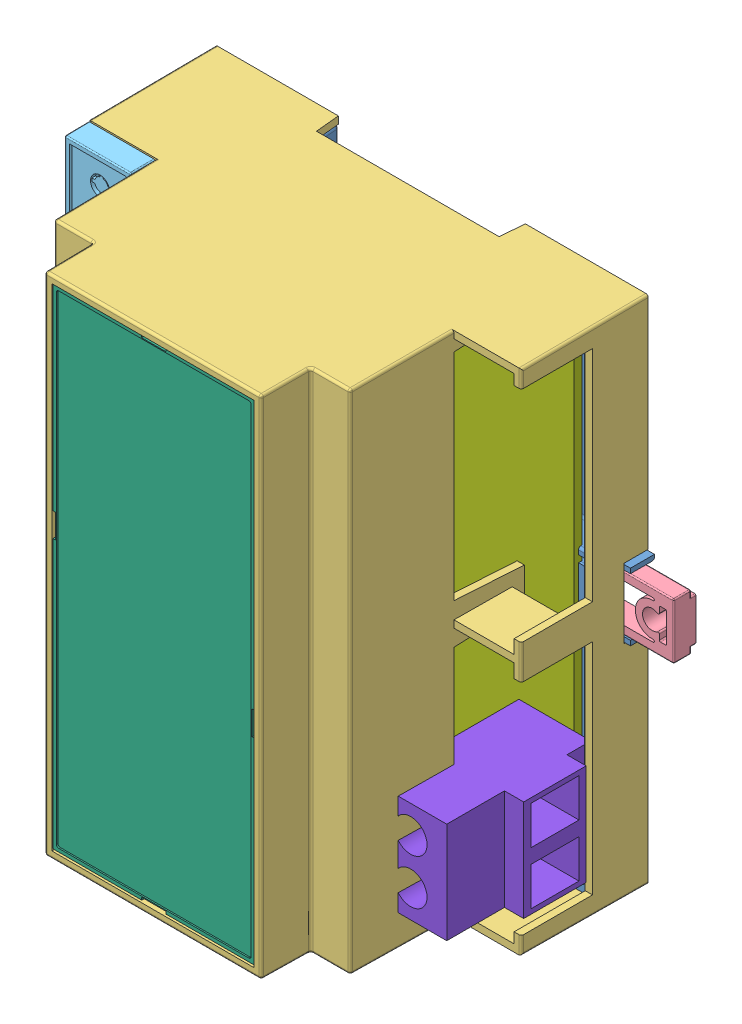
SolidWorks assembly Счетчик для маховика, сборка, configuration Default. Lengths in mm.
Overall size (109.14 106.24 58.15).
13 component instances, 8 part files, 10 mates.
Components (placement in the parent):
- 6 din box-1: 6 din box [Default] at origin size (109.14 106.24 58.15)
  - CNMB-6-Base-1.STEP-1: CNMB-6-Base-1.STEP [Default] at (72.4133 -37.4776 -1.5362) x (0 0 -1) z (-1 0 0) size (10.08 104.2 91.1)
  - CNMB-CW-1.STEP-1: CNMB-CW-1.STEP [Default] at (-24.9867 28.2255 -1.5211) x (-1 0 0) z (0 0 -1) size (31.75 10.57 6.05)
  - CNMB-6-2-Top-1.STEP-1: CNMB-6-2-Top-1.STEP [Default] at (-16.7867 -11.8228 16.8903) size (90 106.24 58.07)
  - CNMB-CW-1.STEP-2: CNMB-CW-1.STEP [Default] at (-25 -32.3717 -1.5388) x (-1 0 0) z (0 0 -1) size (31.75 10.57 6.05)
  - CNMB-CB-1.STEP-1: CNMB-CB-1.STEP [Default] at (83.5178 31.9408 -1.341) x (1 0 0) z (0 0 -1) size (33.1 11.85 5.73)
  - CNMB-3-TG508P.STEP-1: CNMB-3-TG508P.STEP [Default] at (73.2133 67.9724 24.8638) x (0 0 1) z (1 0 0) size (19.8 52.6 14.8)
  - CNMB-3-TG508P.STEP-2: CNMB-3-TG508P.STEP [Default] at (-16.7867 15.692 24.8638) x (0 0 1) z (-1 0 0) size (19.8 52.6 14.8) (hidden)
  - CNMB-3-TG508P.STEP-3: CNMB-3-TG508P.STEP [Default] at (73.2133 15.2224 24.8638) x (0 0 1) z (1 0 0) size (19.8 52.6 14.8)
  - CNMB-3-TG508P.STEP-4: CNMB-3-TG508P.STEP [Default] at (-16.7867 -37.058 24.8638) x (0 0 1) z (-1 0 0) size (19.8 52.6 14.8) (hidden)
  - CNMB-6-PG.STEP-1: CNMB-6-PG.STEP [Default] at (12.0136 -4.007 53.9638) size (42.3 102.2 5.1)
- Плата счетчика маховика-1: Плата счетчика маховика [Default] at (72.4133 -37.4776 4.7638) x (-1 0 0) z (0 0 1) size (75 95 1.6)
- TL800-02-1: TL800-02 [По умолчанию] at (61.7133 -20.3839 21.3638) x (0 1 0) z (1 0 0) size (21 34 19)
Mates (geometry in assembly coordinates):
- InPlace1: in place: plane of ? through (-30.4061 -28.6545 -0.377) normal (0 0 1); plane of ? through (0 0 -0.377) normal (0 0 1); moOrthogonalPlaneRef_w of ? through (-30.4061 -28.6545 -0.377) normal (0 0 1); plane of ? through (0 0 -0.377) normal (0 1 0); plane of ? through (-30.4061 -28.6545 -0.377) normal (0 0 1); plane of ? through (0 0 -0.377) normal (1 0 0); plane of 6 din box-1/CNMB-6-Base-1.STEP-1 through (55.655 -24.6359 4.7638) normal (0 0 1); unknown of Плата счетчика маховика-1
- Coincident1: coincident aligned: plane of 6 din box-1/CNMB-6-Base-1.STEP-1; plane of Плата счетчика маховика-1
- Coincident2: coincident aligned: moOrthogonalPlaneRef_w of 6 din box-1/CNMB-6-Base-1.STEP-1 through (72.4133 -37.4776 4.7638) normal (0 -1 0); plane of Плата счетчика маховика-1 through (72.4133 -37.4776 4.7638) normal (0 -1 0)
- Coincident3: coincident anti-aligned: moOrthogonalPlaneRef_w of 6 din box-1/CNMB-6-Base-1.STEP-1 through (72.4133 -37.4776 4.7638) normal (1 0 0); plane of Плата счетчика маховика-1 through (72.4133 -37.4776 4.7638) normal (-1 0 0)
- Coincident4: coincident anti-aligned: plane of Плата счетчика маховика-1 through (72.4133 -37.4776 6.3638) normal (0 0 1); plane of TL800-02-1 through (61.7133 -9.8839 6.3638) normal (0 0 -1)
- Coincident5: coincident aligned: plane of 6 din box-1 through (0 0 0) normal (0 0 1)
- Coincident6: coincident aligned: plane of 6 din box-1 through (0 0 0) normal (0 1 0)
- Coincident7: coincident aligned: plane of 6 din box-1 through (0 0 0) normal (1 0 0)
- Parallel1: parallel aligned: plane of Плата счетчика маховика-1 through (65.7133 -32.0776 6.3638) normal (0 -1 0); plane of TL800-02-1 through (61.7133 -30.8839 21.3638) normal (0 -1 0)
- Coincident8: coincident aligned: plane of 6 din box-1/CNMB-6-2-Top-1.STEP-1 through (73.2133 -37.1775 24.3638) normal (1 0 0); plane of TL800-02-1 through (73.2133 -9.8839 21.3638) normal (1 0 0)
